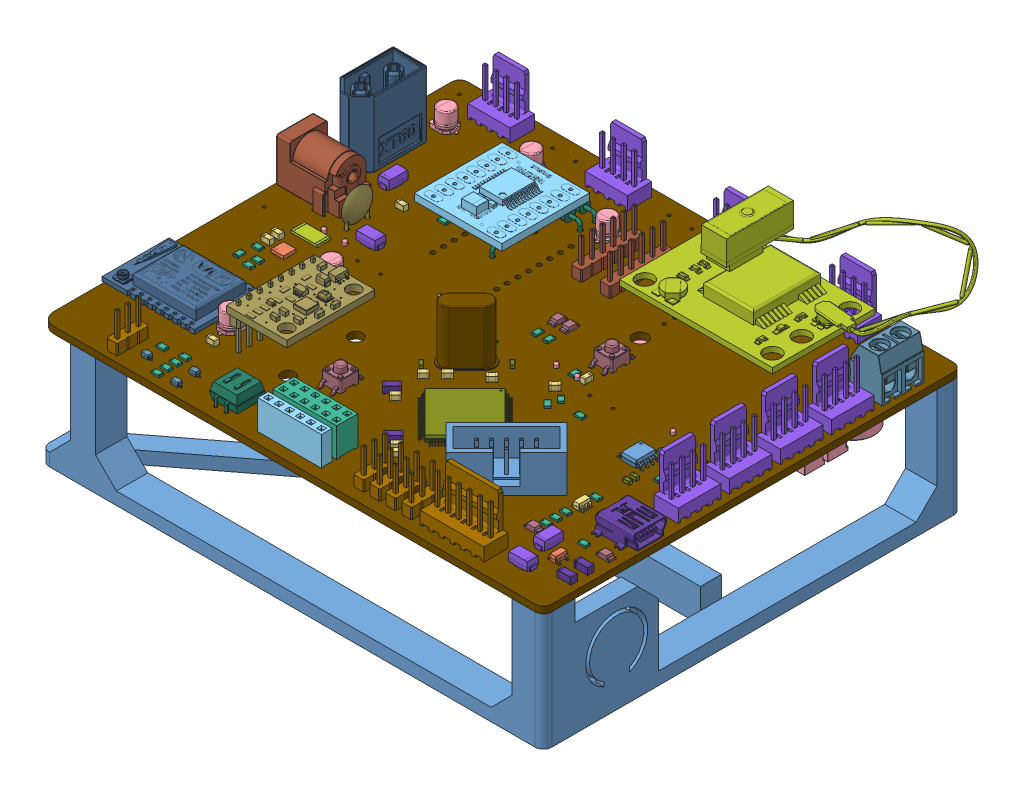
SolidWorks assembly MóduloPCB, configuration Default. Lengths in mm.
Overall size (125.96 62.26 104.91).
242 component instances, 37 part files, 3 mates.
Components (placement in the parent):
- noah_v02-1: noah_v02 [Default] at (-79.7076 93.1619 -169.3417) x (1 0 0) z (0 1 0) size (125.96 104.91 49.76)
  - noah_v02.step-1: noah_v02.step [Default] at origin size (125.96 104.91 49.76)
    - IDC-Header_2x05_P2.54mm_Vertical.step-1: IDC-Header_2x05_P2.54mm_Vertical.step [Default] at (176.6 -132.6 1.65) x (-0.707107 0.707107 0) z (0 0 1) size (9.1 20.36 12.1)
      - SOLID.step-1: SOLID.step [Default] at origin size (9.1 20.36 12.1)
    - DFN-8-1EP_3x3mm_P0.5mm_EP1.66x2.38mm.step-1: DFN-8-1EP_3x3mm_P0.5mm_EP1.66x2.38mm.step [Default] at (105.305 -107.385 1.65) x (0 1 0) z (0 0 1) size (3 2.98 0.77)
      - SOLID-0.step-1: SOLID-0.step [Default] at origin size (3 2.98 0.77)
    - C_0805_2012Metric.step-1: C_0805_2012Metric.step [Default] at (160.4 -70.1 1.65) x (0 -1 0) z (0 0 1) size (2 1.25 1.25)
      - SOLID-1.step-1: SOLID-1.step [Default] at origin size (2 1.25 1.25)
    - CP_Elec_4x4.5.step-1: CP_Elec_4x4.5.step [Default] at (140.6 -65.3 1.65) x (0 -1 0) z (0 0 1) size (5.74 5.46 4.5)
      - SOLID-2.step-1: SOLID-2.step [Default] at origin size (5.74 5.46 4.5)
    - C_0805_2012Metric.step-2: C_0805_2012Metric.step [Default] at (115.6 -134.6 1.65) size (2 1.25 1.25)
      - SOLID-1.step-1: SOLID-1.step [Default] at origin size (2 1.25 1.25)
    - CP_Elec_4x4.5.step-2: CP_Elec_4x4.5.step [Default] at (114.6 -129.4 1.65) x (0 1 0) z (0 0 1) size (5.74 5.46 4.5)
      - SOLID-2.step-1: SOLID-2.step [Default] at origin size (5.74 5.46 4.5)
    - PinSocket_1x06_P2.54mm_Vertical.step-1: PinSocket_1x06_P2.54mm_Vertical.step [Default] at (153.2 -146.2 1.65) x (0 -1 0) z (0 0 1) size (2.54 15.24 10.1)
      - SOLID-3.step-1: SOLID-3.step [Default] at origin size (2.54 15.24 10.1)
    - PinSocket_2x06_P2.54mm_Vertical.step-1: PinSocket_2x06_P2.54mm_Vertical.step [Default] at (153.2 -142.6 1.65) x (0 -1 0) z (0 0 1) size (5.08 15.24 10.1)
      - SOLID-4.step-1: SOLID-4.step [Default] at origin size (5.08 15.24 10.1)
    - ublox_NEO-6M.step-1: ublox_NEO-6M.step [Default] at (181.8 -59.6 11.65) x (0 1 0) z (1 0 0) size (39.06 22.61 48.01)
      - COMPOUND.step-1: COMPOUND.step [Default] at origin size (39.06 22.61 48.01)
    - D_SMA.step-1: D_SMA.step [Default] at (198.4 -143.2 1.65) x (-1 0 0) z (0 0 1) size (5 2.7 2.22)
      - SOLID-5.step-1: SOLID-5.step [Default] at origin size (5 2.7 2.22)
    - PinHeader_1x03_P2.54mm_Vertical.step-1: PinHeader_1x03_P2.54mm_Vertical.step [Default] at (105.6 -147.4 1.65) x (-1 0 0) z (0 0 1) size (2.54 7.62 11.54)
      - SOLID-6.step-1: SOLID-6.step [Default] at origin size (2.54 7.62 11.54)
    - C_0805_2012Metric.step-3: C_0805_2012Metric.step [Default] at (101.3 -107.1 1.65) x (-1 0 0) z (0 0 1) size (2 1.25 1.25)
      - SOLID-1.step-1: SOLID-1.step [Default] at origin size (2 1.25 1.25)
    - C_0805_2012Metric.step-4: C_0805_2012Metric.step [Default] at (101.3 -104.8 1.65) x (-1 0 0) z (0 0 1) size (2 1.25 1.25)
      - SOLID-1.step-1: SOLID-1.step [Default] at origin size (2 1.25 1.25)
    - ESP07.step-1: ESP07.step [Default] at (101.6 -127.3 1.65) x (0 1 0) z (1 0 0) size (19.34 14.61 27.24)
      - COMPOUND-7.step-1: COMPOUND-7.step [Default] at origin size (19.34 14.61 27.24)
    - Power_Barrel_Connector_Jack_694106301002.step-1: Power_Barrel_Connector_Jack_694106301002.step [Default] at (104.13 -90.01 1.65) x (0 -1 0) z (0 0 1) size (9.49 14.48 14.52)
      - COMPOUND-8.step-1: COMPOUND-8.step [Default] at origin size (9.49 14.48 14.52)
    - GY-91.step-1: GY-91.step [Default] at (119 -134.7 9.65) size (14.4 21 11.75)
      - COMPOUND-9.step-1: COMPOUND-9.step [Default] at origin size (14.4 21 11.75)
    - Tact_Switch_4.5mm_SMT.step-1: Tact_Switch_4.5mm_SMT.step [Default] at (139.14 -127.61 1.65) x (0 1 0) z (0 0 1) size (7.5 4.5 4.2)
      - COMPOUND-10.step-1: COMPOUND-10.step [Default] at origin size (7.5 4.5 4.2)
    - Tact_Switch_4.5mm_SMT.step-2: Tact_Switch_4.5mm_SMT.step [Default] at (167.3 -90.93 1.65) x (0 -1 0) z (0 0 1) size (7.5 4.5 4.2)
      - COMPOUND-10.step-1: COMPOUND-10.step [Default] at origin size (7.5 4.5 4.2)
    - tb5p-2p_p5_l10_w7-6_h10.step-1: tb5p-2p_p5_l10_w7-6_h10.step [Default] at (205.55 -62.68 6.65) x (0 1 0) z (1 0 0) size (10.6 14.1 7.6)
      - COMPOUND-11.step-1: COMPOUND-11.step [Default] at origin size (10.6 14.1 7.6)
    - SW_DIP_SPSTx02_Slide_6.7x6.64mm_W7.62mm_P2.54mm_LowProfile.step-1: SW_DIP_SPSTx02_Slide_6.7x6.64mm_W7.62mm_P2.54mm_LowProfile.step [Default] at (131.45 -139.55 1.65) x (-1 0 0) z (0 0 1) size (6.64 7.82 6)
      - SOLID-12.step-1: SOLID-12.step [Default] at origin size (6.64 7.82 6)
    - LQFP-100_14x14mm_P0.5mm.step-1: LQFP-100_14x14mm_P0.5mm.step [Default] at (161.4 -120.1 1.65) x (0.707107 -0.707107 0) z (0 0 1) size (16 16 1.5)
      - SOLID-13.step-1: SOLID-13.step [Default] at origin size (16 16 1.5)
    - USB_Mini-B_Lumberg_2486_01_Horizontal.step-1: USB_Mini-B_Lumberg_2486_01_Horizontal.step [Default] at (203.6 -123.9 1.65) x (0 1 0) z (0 0 1) size (9.9 9.21 5)
      - SOLID-14.step-1: SOLID-14.step [Default] at origin size (9.9 9.21 5)
    - Crystal_HC49-U_Vertical.step-1: Crystal_HC49-U_Vertical.step [Default] at (151.7 -106.6 1.65) x (-0.707107 -0.707107 0) z (0 0 1) size (10.9 4.65 16)
      - SOLID-15.step-1: SOLID-15.step [Default] at origin size (10.9 4.65 16)
    - SOIC-8_3.9x4.9mm_P1.27mm.step-1: SOIC-8_3.9x4.9mm_P1.27mm.step [Default] at (190.4 -107.7 1.65) size (6 4.9 1.75)
      - SOLID-16.step-1: SOLID-16.step [Default] at origin size (6 4.9 1.75)
    - SOT-23-5.step-1: SOT-23-5.step [Default] at (201.6 -138 1.65) size (2.8 2.9 1.55)
      - SOLID-17.step-1: SOLID-17.step [Default] at origin size (2.8 2.9 1.55)
    - SOT-23-6.step-1: SOT-23-6.step [Default] at (193.5 -124.3 1.65) size (2.8 2.9 1.55)
      - SOLID-18.step-1: SOLID-18.step [Default] at origin size (2.8 2.9 1.55)
    - XL4015_StepDown_DC-DC_5A_(CC-CV)_v1.step-1: XL4015_StepDown_DC-DC_5A_(CC-CV)_v1.step [Default] at (119.3 -102.3 -0.05) x (0 1 0) z (0 0 -1) size (51 26 18.15)
      - COMPOUND-19.step-1: COMPOUND-19.step [Default] at origin size (51 26 18.15)
    - XL4015_StepDown_DC-DC_5A_(CC-CV)_v1.step-2: XL4015_StepDown_DC-DC_5A_(CC-CV)_v1.step [Default] at (147.1 -102.4 -0.05) x (0 1 0) z (0 0 -1) size (51 26 18.15)
      - COMPOUND-19.step-1: COMPOUND-19.step [Default] at origin size (51 26 18.15)
    - XL4015_StepDown_DC-DC_5A_(CC-CV)_v1.step-3: XL4015_StepDown_DC-DC_5A_(CC-CV)_v1.step [Default] at (174.9 -102.3 -0.05) x (0 1 0) z (0 0 -1) size (51 26 18.15)
      - COMPOUND-19.step-1: COMPOUND-19.step [Default] at origin size (51 26 18.15)
    - XL4015_StepDown_DC-DC_5A_(CC-CV)_v1.step-4: XL4015_StepDown_DC-DC_5A_(CC-CV)_v1.step [Default] at (91.5 -102.3 -0.05) x (0 1 0) z (0 0 -1) size (51 26 18.15)
      - COMPOUND-19.step-1: COMPOUND-19.step [Default] at origin size (51 26 18.15)
    - TB6612FNG_Motor_Driver.step-1: TB6612FNG_Motor_Driver.step [Default] at (130.68 -80.59 11.65) x (0 0 1) z (1 0 0) size (3.57 20.98 20.9)
      - SOLID-20.step-1: SOLID-20.step [Default] at origin size (3.57 20.98 20.9)
    - R_0805_2012Metric.step-1: R_0805_2012Metric.step [Default] at (168.4 -107.4 1.65) x (0.707107 -0.707107 0) z (0 0 1) size (2 1.2 0.45)
      - SOLID-21.step-1: SOLID-21.step [Default] at origin size (2 1.2 0.45)
    - R_0805_2012Metric.step-2: R_0805_2012Metric.step [Default] at (200.7 -105.4 1.65) x (0 1 0) z (0 0 1) size (2 1.2 0.45)
      - SOLID-21.step-1: SOLID-21.step [Default] at origin size (2 1.2 0.45)
    - R_0805_2012Metric.step-3: R_0805_2012Metric.step [Default] at (200.7 -109.4 1.65) x (0 -1 0) z (0 0 1) size (2 1.2 0.45)
      - SOLID-21.step-1: SOLID-21.step [Default] at origin size (2 1.2 0.45)
    - R_0805_2012Metric.step-4: R_0805_2012Metric.step [Default] at (197.3 -105.4 1.65) x (0 1 0) z (0 0 1) size (2 1.2 0.45)
      - SOLID-21.step-1: SOLID-21.step [Default] at origin size (2 1.2 0.45)
    - R_0805_2012Metric.step-5: R_0805_2012Metric.step [Default] at (197.3 -109.4 1.65) x (0 -1 0) z (0 0 1) size (2 1.2 0.45)
      - SOLID-21.step-1: SOLID-21.step [Default] at origin size (2 1.2 0.45)
    - R_0805_2012Metric.step-6: R_0805_2012Metric.step [Default] at (192.1 -103.5 1.65) size (2 1.2 0.45)
      - SOLID-21.step-1: SOLID-21.step [Default] at origin size (2 1.2 0.45)
    - R_0805_2012Metric.step-7: R_0805_2012Metric.step [Default] at (201.6 -131.9 1.65) x (-1 0 0) z (0 0 1) size (2 1.2 0.45)
      - SOLID-21.step-1: SOLID-21.step [Default] at origin size (2 1.2 0.45)
    - R_0805_2012Metric.step-8: R_0805_2012Metric.step [Default] at (193.5 -120.9 1.65) size (2 1.2 0.45)
      - SOLID-21.step-1: SOLID-21.step [Default] at origin size (2 1.2 0.45)
    - R_0805_2012Metric.step-9: R_0805_2012Metric.step [Default] at (192.9 -127.5 1.65) x (-1 0 0) z (0 0 1) size (2 1.2 0.45)
      - SOLID-21.step-1: SOLID-21.step [Default] at origin size (2 1.2 0.45)
    - R_0805_2012Metric.step-10: R_0805_2012Metric.step [Default] at (192.9 -129.9 1.65) size (2 1.2 0.45)
      - SOLID-21.step-1: SOLID-21.step [Default] at origin size (2 1.2 0.45)
    - R_0805_2012Metric.step-11: R_0805_2012Metric.step [Default] at (110.6 -141.6 1.65) size (2 1.2 0.45)
      - SOLID-21.step-1: SOLID-21.step [Default] at origin size (2 1.2 0.45)
    - R_0805_2012Metric.step-12: R_0805_2012Metric.step [Default] at (177.2 -71.9 1.65) x (-1 0 0) z (0 0 1) size (2 1.2 0.45)
      - SOLID-21.step-1: SOLID-21.step [Default] at origin size (2 1.2 0.45)
    - R_0805_2012Metric.step-13: R_0805_2012Metric.step [Default] at (177.2 -65.3 1.65) x (-1 0 0) z (0 0 1) size (2 1.2 0.45)
      - SOLID-21.step-1: SOLID-21.step [Default] at origin size (2 1.2 0.45)
    - R_0805_2012Metric.step-14: R_0805_2012Metric.step [Default] at (177.2 -69.7 1.65) x (-1 0 0) z (0 0 1) size (2 1.2 0.45)
      - SOLID-21.step-1: SOLID-21.step [Default] at origin size (2 1.2 0.45)
    - R_0805_2012Metric.step-15: R_0805_2012Metric.step [Default] at (177.2 -67.5 1.65) x (-1 0 0) z (0 0 1) size (2 1.2 0.45)
      - SOLID-21.step-1: SOLID-21.step [Default] at origin size (2 1.2 0.45)
    - R_0805_2012Metric.step-16: R_0805_2012Metric.step [Default] at (165.3 -97.8 1.65) x (0 1 0) z (0 0 1) size (2 1.2 0.45)
      - SOLID-21.step-1: SOLID-21.step [Default] at origin size (2 1.2 0.45)
    - R_0805_2012Metric.step-17: R_0805_2012Metric.step [Default] at (152.4 -93.8 1.65) x (0 -1 0) z (0 0 1) size (2 1.2 0.45)
      - SOLID-21.step-1: SOLID-21.step [Default] at origin size (2 1.2 0.45)
    - R_0805_2012Metric.step-18: R_0805_2012Metric.step [Default] at (155.2 -93.8 1.65) x (0 -1 0) z (0 0 1) size (2 1.2 0.45)
      - SOLID-21.step-1: SOLID-21.step [Default] at origin size (2 1.2 0.45)
    - R_0805_2012Metric.step-19: R_0805_2012Metric.step [Default] at (192.9 -132.2 1.65) x (-1 0 0) z (0 0 1) size (2 1.2 0.45)
      - SOLID-21.step-1: SOLID-21.step [Default] at origin size (2 1.2 0.45)
    - R_0805_2012Metric.step-20: R_0805_2012Metric.step [Default] at (169 -104.8 1.65) x (0.707107 -0.707107 0) z (0 0 1) size (2 1.2 0.45)
      - SOLID-21.step-1: SOLID-21.step [Default] at origin size (2 1.2 0.45)
    - R_0805_2012Metric.step-21: R_0805_2012Metric.step [Default] at (174.7 -105.9 1.65) size (2 1.2 0.45)
      - SOLID-21.step-1: SOLID-21.step [Default] at origin size (2 1.2 0.45)
    - R_0805_2012Metric.step-22: R_0805_2012Metric.step [Default] at (111.4 -74.4 1.65) x (0 1 0) z (0 0 1) size (2 1.2 0.45)
      - SOLID-21.step-1: SOLID-21.step [Default] at origin size (2 1.2 0.45)
    - R_0805_2012Metric.step-23: R_0805_2012Metric.step [Default] at (110.4 -77.6 1.65) x (-1 0 0) z (0 0 1) size (2 1.2 0.45)
      - SOLID-21.step-1: SOLID-21.step [Default] at origin size (2 1.2 0.45)
    - R_0805_2012Metric.step-24: R_0805_2012Metric.step [Default] at (101.3 -109.5 1.65) size (2 1.2 0.45)
      - SOLID-21.step-1: SOLID-21.step [Default] at origin size (2 1.2 0.45)
    - R_0805_2012Metric.step-25: R_0805_2012Metric.step [Default] at (100.5 -113.1 1.65) x (0 -1 0) z (0 0 1) size (2 1.2 0.45)
      - SOLID-21.step-1: SOLID-21.step [Default] at origin size (2 1.2 0.45)
    - R_0805_2012Metric.step-26: R_0805_2012Metric.step [Default] at (115.4 -147.6 1.65) size (2 1.2 0.45)
      - SOLID-21.step-1: SOLID-21.step [Default] at origin size (2 1.2 0.45)
    - R_0805_2012Metric.step-27: R_0805_2012Metric.step [Default] at (115.4 -145.4 1.65) size (2 1.2 0.45)
      - SOLID-21.step-1: SOLID-21.step [Default] at origin size (2 1.2 0.45)
    - R_0805_2012Metric.step-28: R_0805_2012Metric.step [Default] at (115.4 -143.2 1.65) size (2 1.2 0.45)
      - SOLID-21.step-1: SOLID-21.step [Default] at origin size (2 1.2 0.45)
    - R_0805_2012Metric.step-29: R_0805_2012Metric.step [Default] at (115.4 -141 1.65) size (2 1.2 0.45)
      - SOLID-21.step-1: SOLID-21.step [Default] at origin size (2 1.2 0.45)
    - R_2512_6332Metric.step-1: R_2512_6332Metric.step [Default] at (105.2 -100.8 1.65) size (6.3 3.2 0.6)
      - SOLID-22.step-1: SOLID-22.step [Default] at origin size (6.3 3.2 0.6)
    - R_0805_2012Metric.step-30: R_0805_2012Metric.step [Default] at (104 -112.2 1.65) x (-1 0 0) z (0 0 1) size (2 1.2 0.45)
      - SOLID-21.step-1: SOLID-21.step [Default] at origin size (2 1.2 0.45)
    - R_0805_2012Metric.step-31: R_0805_2012Metric.step [Default] at (104 -114.4 1.65) x (-1 0 0) z (0 0 1) size (2 1.2 0.45)
      - SOLID-21.step-1: SOLID-21.step [Default] at origin size (2 1.2 0.45)
    - R_0805_2012Metric.step-32: R_0805_2012Metric.step [Default] at (118.1 -81.9 1.65) x (-1 0 0) z (0 0 1) size (2 1.2 0.45)
      - SOLID-21.step-1: SOLID-21.step [Default] at origin size (2 1.2 0.45)
    - Molex_KK-254_AE-6410-04A_1x04_P2.54mm_Vertical.step-1: Molex_KK-254_AE-6410-04A_1x04_P2.54mm_Vertical.step [Default] at (205.6 -95.2 1.65) x (0 -1 0) z (0 0 1) size (10.16 5.8 15.26)
      - SOLID-23.step-1: SOLID-23.step [Default] at origin size (10.16 5.8 15.26)
    - Molex_KK-254_AE-6410-06A_1x06_P2.54mm_Vertical.step-1: Molex_KK-254_AE-6410-06A_1x06_P2.54mm_Vertical.step [Default] at (192 -144.6 1.65) x (-1 0 0) z (0 0 1) size (15.24 5.8 15.26)
      - SOLID-24.step-1: SOLID-24.step [Default] at origin size (15.24 5.8 15.26)
    - Molex_KK-254_AE-6410-04A_1x04_P2.54mm_Vertical.step-2: Molex_KK-254_AE-6410-04A_1x04_P2.54mm_Vertical.step [Default] at (205.6 -70.8 1.65) x (0 -1 0) z (0 0 1) size (10.16 5.8 15.26)
      - SOLID-23.step-1: SOLID-23.step [Default] at origin size (10.16 5.8 15.26)
    - Molex_KK-254_AE-6410-04A_1x04_P2.54mm_Vertical.step-3: Molex_KK-254_AE-6410-04A_1x04_P2.54mm_Vertical.step [Default] at (205.6 -107.4 1.65) x (0 -1 0) z (0 0 1) size (10.16 5.8 15.26)
      - SOLID-23.step-1: SOLID-23.step [Default] at origin size (10.16 5.8 15.26)
    - Molex_KK-254_AE-6410-04A_1x04_P2.54mm_Vertical.step-4: Molex_KK-254_AE-6410-04A_1x04_P2.54mm_Vertical.step [Default] at (205.6 -83 1.65) x (0 -1 0) z (0 0 1) size (10.16 5.8 15.26)
      - SOLID-23.step-1: SOLID-23.step [Default] at origin size (10.16 5.8 15.26)
    - PinHeader_1x03_P2.54mm_Vertical.step-2: PinHeader_1x03_P2.54mm_Vertical.step [Default] at (163.25 -146.15 1.65) x (-1 0 0) z (0 0 1) size (2.54 7.62 11.54)
      - SOLID-6.step-1: SOLID-6.step [Default] at origin size (2.54 7.62 11.54)
    - PinHeader_1x03_P2.54mm_Vertical.step-3: PinHeader_1x03_P2.54mm_Vertical.step [Default] at (167.05 -146.15 1.65) x (-1 0 0) z (0 0 1) size (2.54 7.62 11.54)
      - SOLID-6.step-1: SOLID-6.step [Default] at origin size (2.54 7.62 11.54)
    - PinHeader_1x03_P2.54mm_Vertical.step-4: PinHeader_1x03_P2.54mm_Vertical.step [Default] at (170.85 -146.15 1.65) x (-1 0 0) z (0 0 1) size (2.54 7.62 11.54)
      - SOLID-6.step-1: SOLID-6.step [Default] at origin size (2.54 7.62 11.54)
    - PinHeader_1x03_P2.54mm_Vertical.step-5: PinHeader_1x03_P2.54mm_Vertical.step [Default] at (174.65 -146.15 1.65) x (-1 0 0) z (0 0 1) size (2.54 7.62 11.54)
      - SOLID-6.step-1: SOLID-6.step [Default] at origin size (2.54 7.62 11.54)
    - Molex_KK-254_AE-6410-04A_1x04_P2.54mm_Vertical.step-5: Molex_KK-254_AE-6410-04A_1x04_P2.54mm_Vertical.step [Default] at (108.5 -54.8 1.65) x (-1 0 0) z (0 0 1) size (10.16 5.8 15.26)
      - SOLID-23.step-1: SOLID-23.step [Default] at origin size (10.16 5.8 15.26)
    - Molex_KK-254_AE-6410-04A_1x04_P2.54mm_Vertical.step-6: Molex_KK-254_AE-6410-04A_1x04_P2.54mm_Vertical.step [Default] at (163.9 -55 1.65) x (-1 0 0) z (0 0 1) size (10.16 5.8 15.26)
      - SOLID-23.step-1: SOLID-23.step [Default] at origin size (10.16 5.8 15.26)
    - XT60_Male_Connector.step-1: XT60_Male_Connector.step [Default] at (95.7 -75.4 17.65) x (0 1 0) z (-1 0 0) size (15.93 20.03 8.13)
      - COMPOUND-25.step-1: COMPOUND-25.step [Default] at origin size (15.93 20.03 8.13)
    - Molex_KK-254_AE-6410-04A_1x04_P2.54mm_Vertical.step-7: Molex_KK-254_AE-6410-04A_1x04_P2.54mm_Vertical.step [Default] at (136.5 -54.8 1.65) x (-1 0 0) z (0 0 1) size (10.16 5.8 15.26)
      - SOLID-23.step-1: SOLID-23.step [Default] at origin size (10.16 5.8 15.26)
    - Molex_KK-254_AE-6410-04A_1x04_P2.54mm_Vertical.step-8: Molex_KK-254_AE-6410-04A_1x04_P2.54mm_Vertical.step [Default] at (191.5 -54.9 1.65) x (-1 0 0) z (0 0 1) size (10.16 5.8 15.26)
      - SOLID-23.step-1: SOLID-23.step [Default] at origin size (10.16 5.8 15.26)
    - PinHeader_1x06_P2.54mm_Vertical.step-1: PinHeader_1x06_P2.54mm_Vertical.step [Default] at (152.6 -76.7 1.65) x (-1 0 0) z (0 0 1) size (2.54 15.24 11.54)
      - SOLID-26.step-1: SOLID-26.step [Default] at origin size (2.54 15.24 11.54)
    - PinHeader_1x06_P2.54mm_Vertical.step-2: PinHeader_1x06_P2.54mm_Vertical.step [Default] at (145.8 -76.74 1.65) x (-1 0 0) z (0 0 1) size (2.54 15.24 11.54)
      - SOLID-26.step-1: SOLID-26.step [Default] at origin size (2.54 15.24 11.54)
    - C_Disc_D7.5mm_W2.5mm_P5.00mm.step-1: C_Disc_D7.5mm_W2.5mm_P5.00mm.step [Default] at (108 -95 1.65) x (0 1 0) z (0 0 1) size (7.5 2.5 9.6)
      - SOLID-27.step-1: SOLID-27.step [Default] at origin size (7.5 2.5 9.6)
    - LED_1206_3216Metric.step-1: LED_1206_3216Metric.step [Default] at (206.8 -131.9 1.65) x (-1 0 0) z (0 0 1) size (3.2 1.6 1.1)
      - SOLID-28.step-1: SOLID-28.step [Default] at origin size (3.2 1.6 1.1)
    - D_SMA.step-2: D_SMA.step [Default] at (197.2 -136 1.65) x (0 1 0) z (0 0 1) size (5 2.7 2.22)
      - SOLID-5.step-1: SOLID-5.step [Default] at origin size (5 2.7 2.22)
    - D_SOD-323.step-1: D_SOD-323.step [Default] at (119.9 -147.5 1.65) size (2.5 1.25 1.1)
      - SOLID-29.step-1: SOLID-29.step [Default] at origin size (2.5 1.25 1.1)
    - D_SMA.step-3: D_SMA.step [Default] at (113.8 -95 1.65) x (-1 0 0) z (0 0 1) size (5 2.7 2.22)
      - SOLID-5.step-1: SOLID-5.step [Default] at origin size (5 2.7 2.22)
    - D_SMA.step-4: D_SMA.step [Default] at (115.8 -75.4 1.65) x (0 1 0) z (0 0 1) size (5 2.7 2.22)
      - SOLID-5.step-1: SOLID-5.step [Default] at origin size (5 2.7 2.22)
    - D_SMA.step-5: D_SMA.step [Default] at (104 -79.9 1.65) x (0 1 0) z (0 0 1) size (5 2.7 2.22)
      - SOLID-5.step-1: SOLID-5.step [Default] at origin size (5 2.7 2.22)
    - LED_1206_3216Metric.step-2: LED_1206_3216Metric.step [Default] at (152.4 -89 1.65) x (0 -1 0) z (0 0 1) size (3.2 1.6 1.1)
      - SOLID-28.step-1: SOLID-28.step [Default] at origin size (3.2 1.6 1.1)
    - LED_1206_3216Metric.step-3: LED_1206_3216Metric.step [Default] at (155.2 -89 1.65) x (0 -1 0) z (0 0 1) size (3.2 1.6 1.1)
      - SOLID-28.step-1: SOLID-28.step [Default] at origin size (3.2 1.6 1.1)
    - LED_1206_3216Metric.step-4: LED_1206_3216Metric.step [Default] at (192.4 -134.7 1.65) size (3.2 1.6 1.1)
      - SOLID-28.step-1: SOLID-28.step [Default] at origin size (3.2 1.6 1.1)
    - D_SOD-323.step-2: D_SOD-323.step [Default] at (110.7 -145.4 1.65) size (2.5 1.25 1.1)
      - SOLID-29.step-1: SOLID-29.step [Default] at origin size (2.5 1.25 1.1)
    - D_SOD-323.step-3: D_SOD-323.step [Default] at (119.9 -143.2 1.65) size (2.5 1.25 1.1)
      - SOLID-29.step-1: SOLID-29.step [Default] at origin size (2.5 1.25 1.1)
    - D_DO-41_SOD81_P10.16mm_Horizontal.step-1: D_DO-41_SOD81_P10.16mm_Horizontal.step [Default] at (131 -83.2 1.65) x (0 1 0) z (0 0 1) size (10.96 2.72 5.71)
      - SOLID-30.step-1: SOLID-30.step [Default] at origin size (10.96 2.72 5.71)
    - D_DO-41_SOD81_P10.16mm_Horizontal.step-2: D_DO-41_SOD81_P10.16mm_Horizontal.step [Default] at (136.1 -67.3 1.65) x (-1 0 0) z (0 0 1) size (10.96 2.72 5.71)
      - SOLID-30.step-1: SOLID-30.step [Default] at origin size (10.96 2.72 5.71)
    - D_DO-41_SOD81_P10.16mm_Horizontal.step-3: D_DO-41_SOD81_P10.16mm_Horizontal.step [Default] at (136.1 -63.7 1.65) x (-1 0 0) z (0 0 1) size (10.96 2.72 5.71)
      - SOLID-30.step-1: SOLID-30.step [Default] at origin size (10.96 2.72 5.71)
    - C_0805_2012Metric.step-5: C_0805_2012Metric.step [Default] at (160.8 -135.8 1.65) x (-0.707107 -0.707107 0) z (0 0 1) size (2 1.25 1.25)
      - SOLID-1.step-1: SOLID-1.step [Default] at origin size (2 1.25 1.25)
    - C_0603_1608Metric.step-1: C_0603_1608Metric.step [Default] at (193.96 -113.92 1.65) x (-1 0 0) z (0 0 1) size (1.6 0.8 0.8)
      - SOLID-31.step-1: SOLID-31.step [Default] at origin size (1.6 0.8 0.8)
    - C_0603_1608Metric.step-2: C_0603_1608Metric.step [Default] at (194 -112.2 1.65) x (-1 0 0) z (0 0 1) size (1.6 0.8 0.8)
      - SOLID-31.step-1: SOLID-31.step [Default] at origin size (1.6 0.8 0.8)
    - C_1206_3216Metric.step-1: C_1206_3216Metric.step [Default] at (206.8 -137.1 1.65) size (3.2 1.6 1.6)
      - SOLID-32.step-1: SOLID-32.step [Default] at origin size (3.2 1.6 1.6)
    - C_1206_3216Metric.step-2: C_1206_3216Metric.step [Default] at (206.8 -141.1 1.65) size (3.2 1.6 1.6)
      - SOLID-32.step-1: SOLID-32.step [Default] at origin size (3.2 1.6 1.6)
    - CP_Elec_4x4.5.step-3: CP_Elec_4x4.5.step [Default] at (116.6 -107.2 1.65) size (5.74 5.46 4.5)
      - SOLID-2.step-1: SOLID-2.step [Default] at origin size (5.74 5.46 4.5)
    - CP_Elec_4x4.5.step-4: CP_Elec_4x4.5.step [Default] at (98.8 -62 1.65) x (-1 0 0) z (0 0 1) size (5.74 5.46 4.5)
      - SOLID-2.step-1: SOLID-2.step [Default] at origin size (5.74 5.46 4.5)
    - C_0805_2012Metric.step-6: C_0805_2012Metric.step [Default] at (110.3 -84.1 1.65) size (2 1.25 1.25)
      - SOLID-1.step-1: SOLID-1.step [Default] at origin size (2 1.25 1.25)
    - CP_Elec_4x4.5.step-5: CP_Elec_4x4.5.step [Default] at (117.6 -60.5 1.65) x (-1 0 0) z (0 0 1) size (5.74 5.46 4.5)
      - SOLID-2.step-1: SOLID-2.step [Default] at origin size (5.74 5.46 4.5)
    - C_0805_2012Metric.step-7: C_0805_2012Metric.step [Default] at (168.1 -97.8 1.65) x (0 1 0) z (0 0 1) size (2 1.25 1.25)
      - SOLID-1.step-1: SOLID-1.step [Default] at origin size (2 1.25 1.25)
    - C_1206_3216Metric.step-3: C_1206_3216Metric.step [Default] at (176.8 -118 1.65) x (0.707107 0.707107 0) z (0 0 1) size (3.2 1.6 1.6)
      - SOLID-32.step-1: SOLID-32.step [Default] at origin size (3.2 1.6 1.6)
    - C_1206_3216Metric.step-4: C_1206_3216Metric.step [Default] at (178.6 -119.9 1.65) x (0.707107 0.707107 0) z (0 0 1) size (3.2 1.6 1.6)
      - SOLID-32.step-1: SOLID-32.step [Default] at origin size (3.2 1.6 1.6)
    - C_1206_3216Metric.step-5: C_1206_3216Metric.step [Default] at (157.3 -133.1 1.65) x (-0.707107 -0.707107 0) z (0 0 1) size (3.2 1.6 1.6)
      - SOLID-32.step-1: SOLID-32.step [Default] at origin size (3.2 1.6 1.6)
    - C_0603_1608Metric.step-3: C_0603_1608Metric.step [Default] at (145.2 -114.4 1.65) x (0.707107 -0.707107 0) z (0 0 1) size (1.6 0.8 0.8)
      - SOLID-31.step-1: SOLID-31.step [Default] at origin size (1.6 0.8 0.8)
    - C_0603_1608Metric.step-4: C_0603_1608Metric.step [Default] at (156.1 -103.5 1.65) x (0.707107 -0.707107 0) z (0 0 1) size (1.6 0.8 0.8)
      - SOLID-31.step-1: SOLID-31.step [Default] at origin size (1.6 0.8 0.8)
    - C_0805_2012Metric.step-8: C_0805_2012Metric.step [Default] at (150.6 -113.5 1.65) x (-0.707107 -0.707107 0) z (0 0 1) size (2 1.25 1.25)
      - SOLID-1.step-1: SOLID-1.step [Default] at origin size (2 1.25 1.25)
    - C_0805_2012Metric.step-9: C_0805_2012Metric.step [Default] at (147.7 -116.4 1.65) x (0.707107 0.707107 0) z (0 0 1) size (2 1.25 1.25)
      - SOLID-1.step-1: SOLID-1.step [Default] at origin size (2 1.25 1.25)
    - C_0805_2012Metric.step-10: C_0805_2012Metric.step [Default] at (156.6 -108.9 1.65) x (-0.707107 -0.707107 0) z (0 0 1) size (2 1.25 1.25)
      - SOLID-1.step-1: SOLID-1.step [Default] at origin size (2 1.25 1.25)
    - C_1206_3216Metric.step-6: C_1206_3216Metric.step [Default] at (146.9 -123.1 1.65) x (-0.707107 -0.707107 0) z (0 0 1) size (3.2 1.6 1.6)
      - SOLID-32.step-1: SOLID-32.step [Default] at origin size (3.2 1.6 1.6)
    - C_0805_2012Metric.step-11: C_0805_2012Metric.step [Default] at (166 -103.2 1.65) x (0.707107 0.707107 0) z (0 0 1) size (2 1.25 1.25)
      - SOLID-1.step-1: SOLID-1.step [Default] at origin size (2 1.25 1.25)
    - C_0805_2012Metric.step-12: C_0805_2012Metric.step [Default] at (148.9 -124.3 1.65) x (0.707107 0.707107 0) z (0 0 1) size (2 1.25 1.25)
      - SOLID-1.step-1: SOLID-1.step [Default] at origin size (2 1.25 1.25)
    - C_0805_2012Metric.step-13: C_0805_2012Metric.step [Default] at (159.2 -134.3 1.65) x (0.707107 0.707107 0) z (0 0 1) size (2 1.25 1.25)
      - SOLID-1.step-1: SOLID-1.step [Default] at origin size (2 1.25 1.25)
    - C_0805_2012Metric.step-14: C_0805_2012Metric.step [Default] at (174.8 -116.6 1.65) x (-0.707107 -0.707107 0) z (0 0 1) size (2 1.25 1.25)
      - SOLID-1.step-1: SOLID-1.step [Default] at origin size (2 1.25 1.25)
    - CP_Elec_4x4.5.step-6: CP_Elec_4x4.5.step [Default] at (117.6 -66.1 1.65) x (-1 0 0) z (0 0 1) size (5.74 5.46 4.5)
      - SOLID-2.step-1: SOLID-2.step [Default] at origin size (5.74 5.46 4.5)
    - COMPOUND-33.step-1: COMPOUND-33.step [Default] at origin size (120 100 1.6)
- PCBM00-1: PCBM00 [Default] at (82.7453 65.1619 -91.8181) size (120 28 100)
Mates (geometry in assembly coordinates):
- Coincident1: coincident aligned: plane of noah_v02-1/noah_v02.step-1/COMPOUND-33.step-1 through (130.2924 93.1619 -21.3417) normal (1 0 0); plane of PCBM00-1 through (130.2924 68.1619 -116.3417) normal (1 0 0)
- Coincident2: coincident anti-aligned: plane of noah_v02-1/noah_v02.step-1/COMPOUND-33.step-1 through (70.355 93.1619 -69.394) normal (0 -1 0); plane of PCBM00-1 through (128.2924 93.1619 -117.3417) normal (0 1 0)
- Coincident3: coincident aligned: plane of noah_v02-1/noah_v02.step-1/COMPOUND-33.step-1 through (128.2924 93.1619 -119.3417) normal (0 0 -1); plane of PCBM00-1 through (122.7924 68.1619 -119.3417) normal (0 0 -1)
